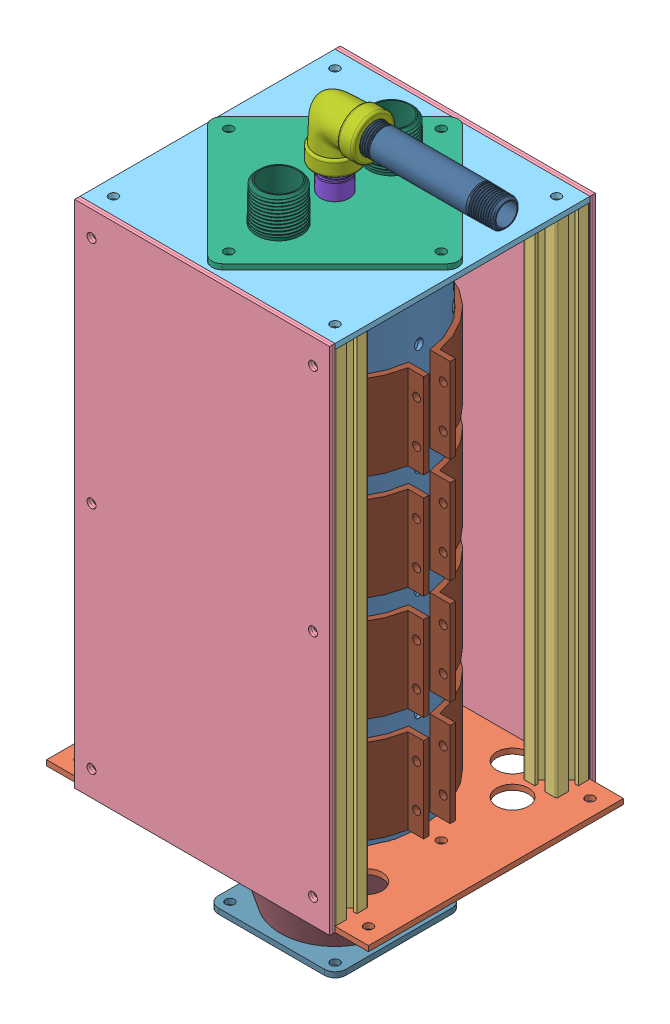
SolidWorks assembly dryer stand alone, configuration Default. Lengths in mm.
Overall size (209.74 423.31 158.7).
25 component instances, 15 part files, 61 mates.
Components (placement in the parent):
- tube-1: tube [Default] at (103.5422 61.3012 185.6839) size (164.34 304.8 101.6)
- flange rev01-1: flange rev01 [Default] at (103.5422 61.3012 185.6839) x (-1 0 0) z (0 0 -1) size (192.4 3.17 152.4)
- HFS5-2020-299-1: HFS5-2020-299 [Default] at (169.7422 63.9262 119.4839) x (-1 0 0) z (0 -1 0) size (20 20 298.45)
- HFS5-2020-299-2: HFS5-2020-299 [Default] at (37.3422 63.9262 119.4839) x (-1 0 0) z (0 -1 0) size (20 20 298.45)
- HFS5-2020-299-3: HFS5-2020-299 [Default] at (169.7422 63.9262 251.8839) x (-1 0 0) z (0 -1 0) size (20 20 298.45)
- HFS5-2020-299-4: HFS5-2020-299 [Default] at (37.3422 363.4762 251.8839) x (-1 0 0) z (0 1 0) size (20 20 298.45)
- side plate 1_16-1: side plate 1_16 [Default] at (103.5422 213.7012 263.4587) x (-1 0 0) z (0 0 -1) size (152.4 304.8 1.57)
- side plate 1_16-2: side plate 1_16 [Default] at (103.5422 213.7012 265.0335) x (-1 0 0) z (0 0 -1) size (152.4 304.8 1.57)
- flange rev02-1: flange rev02 [Default] at (103.5422 362.9262 185.6839) x (-1 0 0) z (0 0 -1) size (152.4 3.17 152.4)
- top cover-1: top cover [Default] at (103.5422 369.2762 185.6839) x (-0.707107 0 -0.707107) z (0 -1 0) size (107.76 107.76 3.17)
- 4452K413_TYPE 316 STAINLESS STL THREADED PIPE FITTING-2: 4452K413_TYPE 316 STAINLESS STL THREADED PIPE FITTING [4452K413] at (103.5422 407.8982 185.6839) x (-1 0 0) z (0 0 1) size (37.28 37.03 30.11)
- 4548K159_STD-WALL TYPE 316-316L SS THRD PIPE NIPPLE-1: 4548K159_STD-WALL TYPE 316-316L SS THRD PIPE NIPPLE [4548K159] at (103.5422 292.6762 185.6839) x (0 1 0) z (0 0 1) size (203.35 17.91 17.78)
- 4464K498_TYPE 304 STAINLESS STL THREADED PIPE FITTING-1: 4464K498_TYPE 304 STAINLESS STL THREADED PIPE FITTING [4464K498] at (103.5422 180.2482 185.6839) x (-0.837169 0 -0.546944) z (0 1 0) size (25.91 25.91 21.03)
- 4548K145_STD-WALL TYPE 316-316L SS THRD PIPE NIPPLE-2: 4548K145_STD-WALL TYPE 316-316L SS THRD PIPE NIPPLE [4548K145] at (161.6142 407.8982 185.6839) x (1 0 0) z (0 -0.851872 -0.523749) size (89.04 17.99 18.06)
- heater band-1: heater band [Default] at (103.5422 257.8762 185.6839) size (116.47 50.8 107.95)
- heater band-2: heater band [Default] at (103.5422 132.2762 185.6839) size (116.47 50.8 107.95)
- heater band-3: heater band [Default] at (103.5422 69.4762 185.6839) size (116.47 50.8 107.95)
- heater band-4: heater band [Default] at (103.5422 195.0762 185.6839) size (116.47 50.8 107.95)
- bottom cover-1: bottom cover [Default] at (103.6306 61.3012 185.6839) x (-0.707107 0 -0.707107) z (0 -1 0) size (107.76 107.76 3.17)
- nozzle reduction-1: nozzle reduction [Default] at (103.6306 61.3012 185.6839) x (-0.837169 0 -0.546944) z (-0.546944 0 0.837169) size (101.6 63.5 101.6)
- 2.5 in bracket-1: 2.5 in bracket [Default] at (103.6306 -2.1988 185.6839) size (76.2 3.17 76.2)
- side plate 1_16-7: side plate 1_16 [Default] at (103.5422 213.7012 107.9091) size (152.4 304.8 1.57)
- side plate 1_16-8: side plate 1_16 [Default] at (103.5422 213.7012 106.3343) size (152.4 304.8 1.57)
- 9157K150_STD-WALL 304-304L SS THRD ONE END PIPE NIPPLE-1: 9157K150_STD-WALL 304-304L SS THRD ONE END PIPE NIPPLE [9157K15] at (103.5422 378.8012 152.0289) x (0 1 0) z (-0.332767 0 0.943009) size (25.49 27.89 27.84)
- 9157K150_STD-WALL 304-304L SS THRD ONE END PIPE NIPPLE-2: 9157K150_STD-WALL 304-304L SS THRD ONE END PIPE NIPPLE [9157K15] at (103.5422 378.8012 219.3389) x (0 1 0) z (-0.546944 0 0.837169) size (25.49 27.89 27.84)
Mates (geometry in assembly coordinates):
- Concentric1: concentric aligned: cylinder of tube-1 through (103.5422 366.1012 185.6839) axis (0 -1 0) radius 50.8; cylinder of flange rev01-1 through (103.5422 64.4762 185.6839) axis (0 -1 0) radius 50.8
- Coincident1: coincident anti-aligned: circle of tube-1; plane of flange rev01-1 through (103.5422 61.3012 185.6839) normal (0 -1 0)
- Coincident2: coincident anti-aligned: plane of flange rev01-1 through (103.5422 64.4762 185.6839) normal (0 1 0); plane of HFS5-2020-299-1 through (178.7422 64.4762 128.4839) normal (0 -1 0)
- Coincident3: coincident aligned: plane of flange rev01-1 through (179.7422 64.4762 109.4839) normal (0 0 -1); plane of HFS5-2020-299-1 through (160.7422 362.9262 109.4839) normal (0 0 -1)
- Coincident5: coincident anti-aligned: plane of flange rev01-1 through (103.5422 64.4762 185.6839) normal (0 1 0); plane of HFS5-2020-299-2 through (46.3422 64.4762 128.4839) normal (0 -1 0)
- Coincident6: coincident aligned: plane of flange rev01-1 through (179.7422 64.4762 109.4839) normal (0 0 -1); plane of HFS5-2020-299-2 through (28.3422 362.9262 109.4839) normal (0 0 -1)
- Coincident8: coincident anti-aligned: plane of flange rev01-1 through (103.5422 64.4762 185.6839) normal (0 1 0); plane of HFS5-2020-299-3 through (178.7422 64.4762 260.8839) normal (0 -1 0)
- Coincident10: coincident aligned: plane of flange rev01-1 through (179.7422 64.4762 261.8839) normal (0 0 1); plane of HFS5-2020-299-3 through (178.7422 362.9262 261.8839) normal (0 0 1)
- Coincident11: coincident anti-aligned: plane of flange rev01-1 through (103.5422 64.4762 185.6839) normal (0 1 0); plane of HFS5-2020-299-4 through (46.3422 64.4762 242.8839) normal (0 -1 0)
- Coincident12: coincident aligned: plane of flange rev01-1 through (179.7422 64.4762 261.8839) normal (0 0 1); plane of HFS5-2020-299-4 through (40.3422 64.4762 261.8839) normal (0 0 1)
- Coincident14: coincident anti-aligned: plane of side plate 1_16-1 through (103.5422 213.7012 263.4587) normal (0 0 1); plane of side plate 1_16-2 through (103.5422 213.7012 263.4587) normal (0 0 -1)
- Coincident15: coincident aligned: plane of side plate 1_16-1 through (179.7422 366.1012 261.8839) normal (0 1 0); plane of side plate 1_16-2 through (179.7422 366.1012 263.4587) normal (0 1 0)
- Coincident16: coincident aligned: plane of side plate 1_16-1 through (179.7422 61.3012 261.8839) normal (1 0 0); plane of side plate 1_16-2 through (179.7422 61.3012 263.4587) normal (1 0 0)
- Coincident17: coincident anti-aligned: plane of HFS5-2020-299-3 through (166.7422 362.9262 261.8839) normal (0 0 1); plane of side plate 1_16-1 through (103.5422 213.7012 261.8839) normal (0 0 -1)
- Coincident18: coincident aligned: plane of flange rev01-1 through (103.5422 61.3012 185.6839) normal (0 -1 0); plane of side plate 1_16-1 through (179.7422 61.3012 261.8839) normal (0 -1 0)
- Coincident19: coincident aligned: plane of HFS5-2020-299-3 through (179.7422 362.9262 254.8839) normal (1 0 0); plane of side plate 1_16-1 through (179.7422 61.3012 261.8839) normal (1 0 0)
- Coincident33: coincident aligned: plane of side plate 1_16-1 through (179.7422 366.1012 261.8839) normal (0 1 0); plane of flange rev02-1 through (103.5422 366.1012 185.6839) normal (0 1 0)
- Coincident34: coincident aligned: plane of HFS5-2020-299-3 through (179.7422 362.9262 254.8839) normal (1 0 0); plane of flange rev02-1 through (179.7422 366.1012 109.4839) normal (1 0 0)
- Coincident35: coincident anti-aligned: plane of side plate 1_16-1 through (103.5422 213.7012 261.8839) normal (0 0 -1); plane of flange rev02-1 through (179.7422 366.1012 261.8839) normal (0 0 1)
- Concentric9: concentric anti-aligned: cylinder of top cover-1 through (103.5422 369.2772 185.6839) axis (0 -1 0) radius 8.5725; cylinder of 4548K159_STD-WALL TYPE 316-316L SS THRD PIPE NIPPLE-1 through (103.5422 292.6762 185.6839) axis (0 1 0) radius 8.5725
- Distance4: distance = 25 mm aligned: plane of 4548K159_STD-WALL TYPE 316-316L SS THRD PIPE NIPPLE-1 through (103.5422 394.2762 185.6839) normal (0 1 0); plane of top cover-1 through (103.5422 369.2762 185.6839) normal (0 1 0)
- Concentric10: concentric aligned: cylinder of 4452K413_TYPE 316 STAINLESS STL THREADED PIPE FITTING-2 through (103.5422 384.2762 185.6839) axis (0 1 0) radius 12.954; cylinder of 4548K159_STD-WALL TYPE 316-316L SS THRD PIPE NIPPLE-1 through (103.5422 292.6762 185.6839) axis (0 1 0) radius 8.5725
- Distance5: distance = 15 mm anti-aligned: plane of 4452K413_TYPE 316 STAINLESS STL THREADED PIPE FITTING-2 through (103.5422 384.2762 185.6839) normal (0 -1 0); plane of top cover-1 through (103.5422 369.2762 185.6839) normal (0 1 0)
- Coincident38: coincident anti-aligned: plane of flange rev02-1 through (103.5422 366.1012 185.6839) normal (0 1 0); plane of top cover-1 through (103.5422 366.1012 185.6839) normal (0 -1 0)
- Concentric11: concentric aligned: cylinder of 4548K159_STD-WALL TYPE 316-316L SS THRD PIPE NIPPLE-1 through (103.5422 292.6762 185.6839) axis (0 1 0) radius 8.5725; cylinder of 4464K498_TYPE 304 STAINLESS STL THREADED PIPE FITTING-1 through (103.5422 195.7422 185.6839) axis (0 1 0) radius 12.954
- Distance6: distance = 10 mm anti-aligned: plane of 4548K159_STD-WALL TYPE 316-316L SS THRD PIPE NIPPLE-1 through (103.5422 191.0762 185.6839) normal (0 -1 0); plane of 4464K498_TYPE 304 STAINLESS STL THREADED PIPE FITTING-1 through (103.5422 201.0762 185.6839) normal (0 1 0)
- Concentric12: concentric anti-aligned: cylinder of 4452K413_TYPE 316 STAINLESS STL THREADED PIPE FITTING-2 through (127.1642 407.8982 185.6839) axis (-1 0 0) radius 12.954; cylinder of 4548K145_STD-WALL TYPE 316-316L SS THRD PIPE NIPPLE-2 through (161.6142 407.8982 185.6839) axis (1 0 0) radius 8.5725
- Distance7: distance = 10 mm anti-aligned: plane of 4548K145_STD-WALL TYPE 316-316L SS THRD PIPE NIPPLE-2 through (117.1642 407.8982 185.6839) normal (-1 0 0); plane of 4452K413_TYPE 316 STAINLESS STL THREADED PIPE FITTING-2 through (127.1642 407.8982 185.6839) normal (1 0 0)
- Concentric13: concentric aligned: cylinder of tube-1 through (103.5422 366.1012 185.6839) axis (0 -1 0) radius 50.8; cylinder of heater band-3 through (103.5422 120.2762 185.6839) axis (0 -1 0) radius 50.8
- Concentric14: concentric aligned: cylinder of tube-1 through (103.5422 366.1012 185.6839) axis (0 -1 0) radius 50.8; cylinder of heater band-2 through (103.5422 183.0762 185.6839) axis (0 -1 0) radius 50.8
- Concentric15: concentric aligned: cylinder of tube-1 through (103.5422 366.1012 185.6839) axis (0 -1 0) radius 50.8; cylinder of heater band-4 through (103.5422 245.8762 185.6839) axis (0 -1 0) radius 50.8
- Concentric16: concentric aligned: cylinder of tube-1 through (103.5422 366.1012 185.6839) axis (0 -1 0) radius 50.8; cylinder of heater band-1 through (103.5422 308.6762 185.6839) axis (0 -1 0) radius 50.8
- Distance8: distance = 5 mm anti-aligned: plane of heater band-3 through (103.5422 69.4762 185.6839) normal (0 -1 0); plane of flange rev01-1 through (103.5422 64.4762 185.6839) normal (0 1 0)
- Distance9: distance = 12 mm anti-aligned: plane of heater band-2 through (103.5422 132.2762 185.6839) normal (0 -1 0); plane of heater band-3 through (103.5422 120.2762 185.6839) normal (0 1 0)
- Distance10: distance = 12 mm anti-aligned: plane of heater band-2 through (103.5422 183.0762 185.6839) normal (0 1 0); plane of heater band-4 through (103.5422 195.0762 185.6839) normal (0 -1 0)
- Distance11: distance = 12 mm anti-aligned: plane of heater band-4 through (103.5422 245.8762 185.6839) normal (0 1 0); plane of heater band-1 through (103.5422 257.8762 185.6839) normal (0 -1 0)
- Coincident49: coincident aligned: plane of heater band-2 through (157.1424 183.0762 176.1589) normal (0 0 -1); plane of heater band-3 through (157.1424 120.2762 176.1589) normal (0 0 -1)
- Coincident50: coincident aligned: plane of heater band-2 through (157.1424 183.0762 176.1589) normal (0 0 -1); plane of heater band-4 through (157.1424 245.8762 176.1589) normal (0 0 -1)
- Coincident51: coincident aligned: plane of heater band-1 through (157.1424 308.6762 176.1589) normal (0 0 -1); plane of heater band-4 through (157.1424 245.8762 176.1589) normal (0 0 -1)
- Parallel5: parallel anti-aligned: plane of HFS5-2020-299-1 through (166.7422 362.9262 129.4839) normal (0 0 1); plane of heater band-3 through (157.1424 120.2762 176.1589) normal (0 0 -1)
- Coincident53: coincident anti-aligned: plane of flange rev01-1 through (103.5422 61.3012 185.6839) normal (0 -1 0); plane of bottom cover-1 through (103.6306 61.3012 185.6839) normal (0 1 0)
- Coincident54: coincident anti-aligned: plane of tube-1 through (103.5422 61.3012 185.6839) normal (0 -1 0); plane of nozzle reduction-1 through (103.6306 61.3012 185.6839) normal (0 1 0)
- Coincident55: coincident aligned: cylinder of bottom cover-1 through (103.6306 61.3022 185.6839) axis (0 -1 0) radius 50.8; circle of nozzle reduction-1
- Coincident56: coincident aligned: circle of nozzle reduction-1; cylinder of 2.5 in bracket-1 through (103.6306 0.9762 185.6839) axis (0 -1 0) radius 31.75
- Coincident57: coincident aligned: plane of nozzle reduction-1 through (103.6306 -2.1988 185.6839) normal (0 -1 0); plane of 2.5 in bracket-1 through (103.6306 -2.1988 185.6839) normal (0 -1 0)
- Parallel6: parallel: line of flange rev01-1 through (199.7422 61.3012 109.4839) axis (-1 0 0); plane of 2.5 in bracket-1 through (65.5306 0.9762 147.5839) normal (0 0 -1)
- Concentric20: concentric aligned: cylinder of tube-1 through (103.5422 366.1012 185.6839) axis (0 -1 0) radius 50.8; cylinder of top cover-1 through (103.5422 369.2772 185.6839) axis (0 -1 0) radius 8.5725
- Angle1: planar angle = 0.785398 rad aligned: plane of top cover-1 through (27.3422 366.1012 185.6839) normal (-0.707107 0 -0.707107); plane of flange rev02-1 through (27.3422 366.1012 109.4839) normal (-1 0 0)
- Coincident73: coincident anti-aligned: plane of side plate 1_16-7 through (103.5422 213.7012 107.9091) normal (0 0 -1); plane of side plate 1_16-8 through (103.5422 213.7012 107.9091) normal (0 0 1)
- Coincident74: coincident aligned: plane of side plate 1_16-7 through (27.3422 61.3012 109.4839) normal (-1 0 0); plane of side plate 1_16-8 through (27.3422 61.3012 107.9091) normal (-1 0 0)
- Coincident75: coincident aligned: plane of side plate 1_16-7 through (27.3422 366.1012 109.4839) normal (0 1 0); plane of side plate 1_16-8 through (27.3422 366.1012 107.9091) normal (0 1 0)
- Coincident76: coincident aligned: plane of flange rev02-1 through (103.5422 366.1012 185.6839) normal (0 1 0); plane of side plate 1_16-7 through (27.3422 366.1012 109.4839) normal (0 1 0)
- Coincident77: coincident anti-aligned: plane of HFS5-2020-299-1 through (160.7422 362.9262 109.4839) normal (0 0 -1); plane of side plate 1_16-7 through (103.5422 213.7012 109.4839) normal (0 0 1)
- Concentric21: concentric anti-aligned: cylinder of top cover-1 through (103.5422 369.2772 152.0289) axis (0 -1 0) radius 13.335; cylinder of 9157K150_STD-WALL 304-304L SS THRD ONE END PIPE NIPPLE-1 through (103.5422 366.1012 152.0289) axis (0 1 0) radius 13.335
- Coincident79: coincident aligned: circle of top cover-1; plane of 9157K150_STD-WALL 304-304L SS THRD ONE END PIPE NIPPLE-1 through (103.5422 366.1012 152.0289) normal (0 -1 0)
- Coincident80: coincident aligned: circle of top cover-1; plane of 9157K150_STD-WALL 304-304L SS THRD ONE END PIPE NIPPLE-2 through (103.5422 366.1012 219.3389) normal (0 -1 0)
- Concentric22: concentric anti-aligned: cylinder of top cover-1 through (103.5422 369.2772 219.3389) axis (0 -1 0) radius 13.335; cylinder of 9157K150_STD-WALL 304-304L SS THRD ONE END PIPE NIPPLE-2 through (103.5422 366.1012 219.3389) axis (0 1 0) radius 13.335
- Parallel10: parallel aligned: plane of side plate 1_16-2 through (103.5422 213.7012 265.0335) normal (0 0 1); plane of 4452K413_TYPE 316 STAINLESS STL THREADED PIPE FITTING-2 through (103.5422 407.8982 185.6839) normal (0 0 1)
- Parallel11: parallel aligned: plane of side plate 1_16-2 through (103.5422 213.7012 265.0335) normal (0 0 1); plane of assembly through (0 0 0) normal (0 0 1)
- Concentric23: concentric anti-aligned: cylinder of flange rev01-1 through (103.5422 61.3002 122.1839) axis (0 1 0) radius 2.665; cylinder of bottom cover-1 through (103.5422 61.3022 122.1839) axis (0 -1 0) radius 2.665
- Concentric24: concentric anti-aligned: cylinder of flange rev01-1 through (167.0422 61.3002 185.6839) axis (0 1 0) radius 2.665; cylinder of bottom cover-1 through (167.0422 61.3022 185.6839) axis (0 -1 0) radius 2.665
